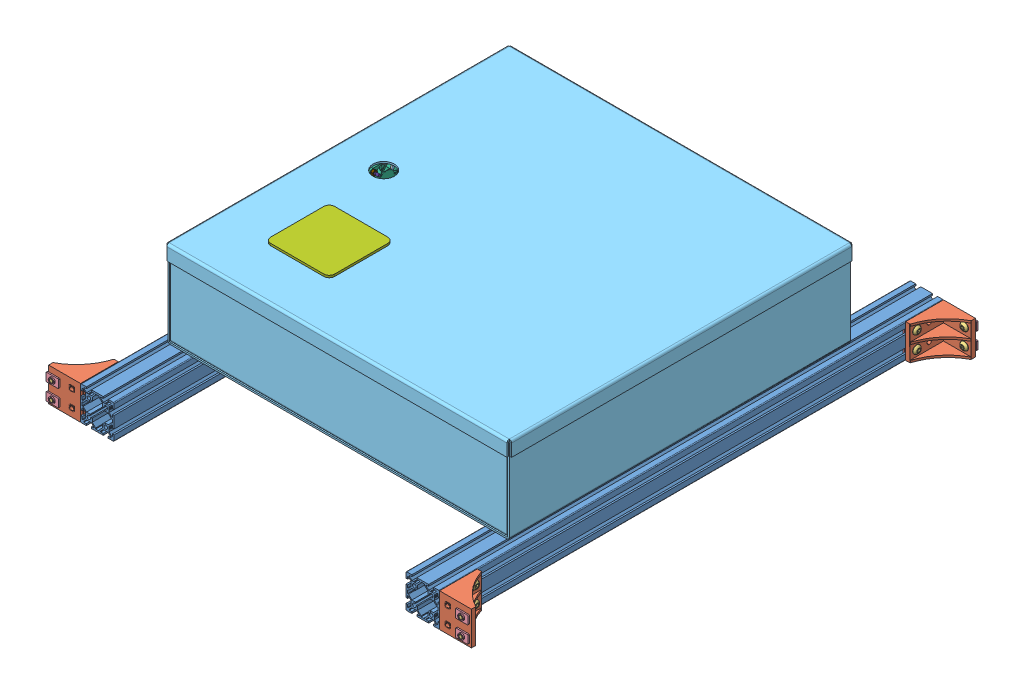
SolidWorks assembly e box uprights, configuration Default. Lengths in mm.
Overall size (503.46 146.17 610.56).
137 component instances, 28 part files, 18 mates.
Components (placement in the parent):
- 4040 600mm-1: 4040 600mm [Default] at (133.4029 328.2364 998.0644) size (40 40 600)
- 4040 600mm-2: 4040 600mm [Default] at (520.8624 328.2364 998.0644) size (40 40 600)
- corner braket assembly-1: corner braket assembly [Default] at (98.8149 314.6768 215.5379) x (0 -1 0) z (-1 0 0) size (40 50.28 43.28)
  - _HBLFSDW5h5_2-1: _HBLFSDW5h5_2 [Default] at (-13.5596 -17.4734 -14.588) size (40 45.8 38.8)
  - 91239A224_CLASS 10.9 STL BUTTON-HEAD SOCKET CAP SCREW-1: 91239A224_CLASS 10.9 STL BUTTON-HEAD SOCKET CAP SCREW [91239A224] at (-23.5596 19.5266 -6.838) size (9.5 9.5 13.21)
  - 91239A224_CLASS 10.9 STL BUTTON-HEAD SOCKET CAP SCREW-3: 91239A224_CLASS 10.9 STL BUTTON-HEAD SOCKET CAP SCREW [91239A224] at (-3.5596 19.5266 -6.838) size (9.5 9.5 13.21)
  - 91239A224_CLASS 10.9 STL BUTTON-HEAD SOCKET CAP SCREW-5: 91239A224_CLASS 10.9 STL BUTTON-HEAD SOCKET CAP SCREW [91239A224] at (-3.5596 -9.7234 15.412) x (1 0 0) z (0 1 0) size (9.5 9.5 13.21)
  - 91239A224_CLASS 10.9 STL BUTTON-HEAD SOCKET CAP SCREW-6: 91239A224_CLASS 10.9 STL BUTTON-HEAD SOCKET CAP SCREW [91239A224] at (-23.5596 -9.7234 15.412) x (1 0 0) z (0 1 0) size (9.5 9.5 13.21)
  - HNKK5-5-2: HNKK5-5 [Default] at (-23.5596 19.5266 -16.588) x (0 0 1) z (0 -1 0) size (3 10 15)
  - HNKK5-5-4: HNKK5-5 [Default] at (-3.5596 19.5266 -16.588) x (0 0 1) z (0 -1 0) size (3 10 15)
  - HNKK5-5-5: HNKK5-5 [Default] at (-23.5596 -19.4734 15.412) x (0 1 0) z (0 0 1) size (3 10 15)
  - HNKK5-5-6: HNKK5-5 [Default] at (-3.5596 -19.4734 15.412) x (0 1 0) z (0 0 1) size (3 10 15)
- corner braket assembly-2: corner braket assembly [Default] at (98.8149 341.796 780.591) x (0 1 0) z (-1 0 0) size (40 50.28 43.28)
  - _HBLFSDW5h5_2-1: _HBLFSDW5h5_2 [Default] at (-13.5596 -17.4734 -14.588) size (40 45.8 38.8)
  - 91239A224_CLASS 10.9 STL BUTTON-HEAD SOCKET CAP SCREW-1: 91239A224_CLASS 10.9 STL BUTTON-HEAD SOCKET CAP SCREW [91239A224] at (-23.5596 19.5266 -6.838) size (9.5 9.5 13.21)
  - 91239A224_CLASS 10.9 STL BUTTON-HEAD SOCKET CAP SCREW-3: 91239A224_CLASS 10.9 STL BUTTON-HEAD SOCKET CAP SCREW [91239A224] at (-3.5596 19.5266 -6.838) size (9.5 9.5 13.21)
  - 91239A224_CLASS 10.9 STL BUTTON-HEAD SOCKET CAP SCREW-5: 91239A224_CLASS 10.9 STL BUTTON-HEAD SOCKET CAP SCREW [91239A224] at (-3.5596 -9.7234 15.412) x (1 0 0) z (0 1 0) size (9.5 9.5 13.21)
  - 91239A224_CLASS 10.9 STL BUTTON-HEAD SOCKET CAP SCREW-6: 91239A224_CLASS 10.9 STL BUTTON-HEAD SOCKET CAP SCREW [91239A224] at (-23.5596 -9.7234 15.412) x (1 0 0) z (0 1 0) size (9.5 9.5 13.21)
  - HNKK5-5-2: HNKK5-5 [Default] at (-23.5596 19.5266 -16.588) x (0 0 1) z (0 -1 0) size (3 10 15)
  - HNKK5-5-4: HNKK5-5 [Default] at (-3.5596 19.5266 -16.588) x (0 0 1) z (0 -1 0) size (3 10 15)
  - HNKK5-5-5: HNKK5-5 [Default] at (-23.5596 -19.4734 15.412) x (0 1 0) z (0 0 1) size (3 10 15)
  - HNKK5-5-6: HNKK5-5 [Default] at (-3.5596 -19.4734 15.412) x (0 1 0) z (0 0 1) size (3 10 15)
- corner braket assembly-3: corner braket assembly [Default] at (555.4504 341.796 215.5379) x (0 1 0) z (1 0 0) size (40 50.28 43.28)
  - _HBLFSDW5h5_2-1: _HBLFSDW5h5_2 [Default] at (-13.5596 -17.4734 -14.588) size (40 45.8 38.8)
  - 91239A224_CLASS 10.9 STL BUTTON-HEAD SOCKET CAP SCREW-1: 91239A224_CLASS 10.9 STL BUTTON-HEAD SOCKET CAP SCREW [91239A224] at (-23.5596 19.5266 -6.838) size (9.5 9.5 13.21)
  - 91239A224_CLASS 10.9 STL BUTTON-HEAD SOCKET CAP SCREW-3: 91239A224_CLASS 10.9 STL BUTTON-HEAD SOCKET CAP SCREW [91239A224] at (-3.5596 19.5266 -6.838) size (9.5 9.5 13.21)
  - 91239A224_CLASS 10.9 STL BUTTON-HEAD SOCKET CAP SCREW-5: 91239A224_CLASS 10.9 STL BUTTON-HEAD SOCKET CAP SCREW [91239A224] at (-3.5596 -9.7234 15.412) x (1 0 0) z (0 1 0) size (9.5 9.5 13.21)
  - 91239A224_CLASS 10.9 STL BUTTON-HEAD SOCKET CAP SCREW-6: 91239A224_CLASS 10.9 STL BUTTON-HEAD SOCKET CAP SCREW [91239A224] at (-23.5596 -9.7234 15.412) x (1 0 0) z (0 1 0) size (9.5 9.5 13.21)
  - HNKK5-5-2: HNKK5-5 [Default] at (-23.5596 19.5266 -16.588) x (0 0 1) z (0 -1 0) size (3 10 15)
  - HNKK5-5-4: HNKK5-5 [Default] at (-3.5596 19.5266 -16.588) x (0 0 1) z (0 -1 0) size (3 10 15)
  - HNKK5-5-5: HNKK5-5 [Default] at (-23.5596 -19.4734 15.412) x (0 1 0) z (0 0 1) size (3 10 15)
  - HNKK5-5-6: HNKK5-5 [Default] at (-3.5596 -19.4734 15.412) x (0 1 0) z (0 0 1) size (3 10 15)
- corner braket assembly-4: corner braket assembly [Default] at (555.4504 314.6768 780.591) x (0 -1 0) z (1 0 0) size (40 50.28 43.28)
  - _HBLFSDW5h5_2-1: _HBLFSDW5h5_2 [Default] at (-13.5596 -17.4734 -14.588) size (40 45.8 38.8)
  - 91239A224_CLASS 10.9 STL BUTTON-HEAD SOCKET CAP SCREW-1: 91239A224_CLASS 10.9 STL BUTTON-HEAD SOCKET CAP SCREW [91239A224] at (-23.5596 19.5266 -6.838) size (9.5 9.5 13.21)
  - 91239A224_CLASS 10.9 STL BUTTON-HEAD SOCKET CAP SCREW-3: 91239A224_CLASS 10.9 STL BUTTON-HEAD SOCKET CAP SCREW [91239A224] at (-3.5596 19.5266 -6.838) size (9.5 9.5 13.21)
  - 91239A224_CLASS 10.9 STL BUTTON-HEAD SOCKET CAP SCREW-5: 91239A224_CLASS 10.9 STL BUTTON-HEAD SOCKET CAP SCREW [91239A224] at (-3.5596 -9.7234 15.412) x (1 0 0) z (0 1 0) size (9.5 9.5 13.21)
  - 91239A224_CLASS 10.9 STL BUTTON-HEAD SOCKET CAP SCREW-6: 91239A224_CLASS 10.9 STL BUTTON-HEAD SOCKET CAP SCREW [91239A224] at (-23.5596 -9.7234 15.412) x (1 0 0) z (0 1 0) size (9.5 9.5 13.21)
  - HNKK5-5-2: HNKK5-5 [Default] at (-23.5596 19.5266 -16.588) x (0 0 1) z (0 -1 0) size (3 10 15)
  - HNKK5-5-4: HNKK5-5 [Default] at (-3.5596 19.5266 -16.588) x (0 0 1) z (0 -1 0) size (3 10 15)
  - HNKK5-5-5: HNKK5-5 [Default] at (-23.5596 -19.4734 15.412) x (0 1 0) z (0 0 1) size (3 10 15)
  - HNKK5-5-6: HNKK5-5 [Default] at (-3.5596 -19.4734 15.412) x (0 1 0) z (0 0 1) size (3 10 15)
- elc box assebly-1: elc box assebly [Default] at (129.7196 154.3271 230.9368) size (410.46 106.17 430.94)
  - Electrical Enclosure 16 in-1: Electrical Enclosure 16 in [Default] at (-5.7869 193.9093 67.1276) size (410.46 103.63 410.46)
  - elc component panel-1: elc component panel [Default] at (423.6423 -1.464 537.2069) x (-1 0 0) z (0 0 -1) size (369.37 85.56 330.2)
    - elc plate-1: elc plate [Default] at (226.2293 207.4053 266.8793) size (368.3 1.59 330.2)
    - power supply with standoffs-1: power supply with standoffs [Default] at (35.6304 133.9192 294.786) x (0 0 -1) z (1 0 0) size (115.2 58.27 215)
      - __-1: __ [По умолчанию] at (110.1067 83.0736 152.0488) size (115.2 50.11 215)
      - 95783A055_NYLON 6 6 MALE-FEMALE THREADED HEX STANDOFF-1: 95783A055_NYLON 6 6 MALE-FEMALE THREADED HEX STANDOFF [95783A055] at (85.1067 81.4236 77.0488) x (0 1 0) z (0 0 1) size (13.03 5.2 4.5)
      - 95783A055_NYLON 6 6 MALE-FEMALE THREADED HEX STANDOFF-2: 95783A055_NYLON 6 6 MALE-FEMALE THREADED HEX STANDOFF [95783A055] at (135.1067 81.4236 77.0488) x (0 1 0) z (-0.939028 0 -0.343839) size (13.03 5.2 4.5)
      - 95783A055_NYLON 6 6 MALE-FEMALE THREADED HEX STANDOFF-3: 95783A055_NYLON 6 6 MALE-FEMALE THREADED HEX STANDOFF [95783A055] at (135.1067 81.4236 227.0488) x (0 1 0) z (-0.996262 0 -0.086381) size (13.03 5.2 4.5)
      - 95783A055_NYLON 6 6 MALE-FEMALE THREADED HEX STANDOFF-4: 95783A055_NYLON 6 6 MALE-FEMALE THREADED HEX STANDOFF [95783A055] at (85.1067 81.4236 227.0488) x (0 1 0) z (-0.990494 0 -0.137554) size (13.03 5.2 4.5)
    - arduino board assembly-1: arduino board assembly [Default] at (260.6228 173.6976 405.5467) x (0 0 -1) z (1 0 0) size (100 30.86 52.88)
      - ArduinoMega2560 CORRECTED-1: ArduinoMega2560 CORRECTED [Default] at (48.9673 43.2952 72.715) size (100 11.65 51.63)
      - breakout board-1: breakout board [Default] at (48.9673 54.2952 72.715) size (100 7 51.63)
      - 95783A055_NYLON 6 6 MALE-FEMALE THREADED HEX STANDOFF-1: 95783A055_NYLON 6 6 MALE-FEMALE THREADED HEX STANDOFF [95783A055] at (84.2031 36.9452 49.5995) x (0 -1 0) z (0 0 1) size (13.03 5.2 4.5)
      - 95783A055_NYLON 6 6 MALE-FEMALE THREADED HEX STANDOFF-2: 95783A055_NYLON 6 6 MALE-FEMALE THREADED HEX STANDOFF [95783A055] at (3.483 36.9452 49.7272) x (0 -1 0) z (0 0 1) size (13.03 5.2 4.5)
      - 95783A055_NYLON 6 6 MALE-FEMALE THREADED HEX STANDOFF-3: 95783A055_NYLON 6 6 MALE-FEMALE THREADED HEX STANDOFF [95783A055] at (9.6911 36.9452 96.9805) x (0 -1 0) z (0 0 1) size (13.03 5.2 4.5)
      - 91290A110_BLACK-OXIDE CLASS 12.9 SOCKET HEAD CAP SCREW-1: 91290A110_BLACK-OXIDE CLASS 12.9 SOCKET HEAD CAP SCREW [91290A110] at (9.6911 39.2952 96.9805) x (1 0 0) z (0 -1 0) size (5.5 5.5 8.18)
      - 91290A110_BLACK-OXIDE CLASS 12.9 SOCKET HEAD CAP SCREW-2: 91290A110_BLACK-OXIDE CLASS 12.9 SOCKET HEAD CAP SCREW [91290A110] at (84.2031 39.2952 49.5995) x (1 0 0) z (0 -1 0) size (5.5 5.5 8.18)
      - 91290A110_BLACK-OXIDE CLASS 12.9 SOCKET HEAD CAP SCREW-3: 91290A110_BLACK-OXIDE CLASS 12.9 SOCKET HEAD CAP SCREW [91290A110] at (3.483 39.2952 49.7272) x (1 0 0) z (0 -1 0) size (5.5 5.5 8.18)
    - din rail assmbly-1: din rail assmbly [Default] at (226.6874 101.8607 473.572) x (-1 0 0) z (0 0 -1) size (90.31 80.69 125)
      - DIN 59_0-1: DIN 59_0 [00] at (103.6081 107.1321 54.2926) size (35 7.5 125)
      - SEIMENS 8WA1 808 DIN RAIL END RETAINER-1: SEIMENS 8WA1 808 DIN RAIL END RETAINER [Default] at (102.6081 107.6321 71.2884) size (45 44.95 10)
      - SEIMENS 8WA1 808 DIN RAIL END RETAINER-3: SEIMENS 8WA1 808 DIN RAIL END RETAINER [Default] at (102.6081 107.6321 162.4924) size (45 44.95 10)
      - 3812830-8: 3812830 [Default] at (102.7638 140.3713 56.6988) x (0 0 -1) z (1 0 0) size (6.2 76.69 90.31)
        - 3812830A-1: 3812830A [Default] at (-75.9936 -29.2392 18.3443) size (6.2 76.69 90.31)
        - 3812830B-1: 3812830B [Default] at (-75.3936 25.9608 19.6) size (5 19.3 28)
      - 3812830-9: 3812830 [Default] at (102.7638 140.3713 62.8988) x (0 0 -1) z (1 0 0) size (6.2 76.69 90.31)
        - 3812830A-1: 3812830A [Default] at (-75.9936 -29.2392 18.3443) size (6.2 76.69 90.31)
        - 3812830B-1: 3812830B [Default] at (-75.3936 25.9608 19.6) size (5 19.3 28)
      - 3812830-10: 3812830 [Default] at (102.7638 140.3713 69.0988) x (0 0 -1) z (1 0 0) size (6.2 76.69 90.31)
        - 3812830A-1: 3812830A [Default] at (-75.9936 -29.2392 18.3443) size (6.2 76.69 90.31)
        - 3812830B-1: 3812830B [Default] at (-75.3936 25.9608 19.6) size (5 19.3 28)
      - 3812830-11: 3812830 [Default] at (102.7638 140.3713 75.2988) x (0 0 -1) z (1 0 0) size (6.2 76.69 90.31)
        - 3812830A-1: 3812830A [Default] at (-75.9936 -29.2392 18.3443) size (6.2 76.69 90.31)
        - 3812830B-1: 3812830B [Default] at (-75.3936 25.9608 19.6) size (5 19.3 28)
      - 3812830-12: 3812830 [Default] at (102.7638 140.3713 81.4988) x (0 0 -1) z (1 0 0) size (6.2 76.69 90.31)
        - 3812830A-1: 3812830A [Default] at (-75.9936 -29.2392 18.3443) size (6.2 76.69 90.31)
        - 3812830B-1: 3812830B [Default] at (-75.3936 25.9608 19.6) size (5 19.3 28)
      - Din fuse-1: Din fuse [Default] at (59.9389 109.5521 90.7664) size (82.55 57.15 9.65)
      - Din fuse-2: Din fuse [Default] at (59.9389 109.5521 81.1144) size (82.55 57.15 9.65)
      - dinrail_Terminal-11: dinrail_Terminal [Default] at (121.1081 114.6321 95.5924) size (48 46.85 5.15)
      - dinrail_Terminal-12: dinrail_Terminal [Default] at (121.1081 114.6321 100.7424) size (48 46.85 5.15)
      - dinrail_Terminal-13: dinrail_Terminal [Default] at (121.1081 114.6321 111.0424) size (48 46.85 5.15)
      - dinrail_Terminal-16: dinrail_Terminal [Default] at (121.1081 114.6321 105.8924) size (48 46.85 5.15)
      - dinrail_Terminal-17: dinrail_Terminal [Default] at (121.1081 114.6321 116.1924) size (48 46.85 5.15)
      - dinrail_Terminal-18: dinrail_Terminal [Default] at (121.1081 114.6321 121.3424) size (48 46.85 5.15)
    - arduino board assembly-2: arduino board assembly [Default] at (164.5922 173.6976 405.5467) x (0 0 -1) z (1 0 0) size (100 30.86 52.88)
      - ArduinoMega2560 CORRECTED-1: ArduinoMega2560 CORRECTED [Default] at (48.9673 43.2952 72.715) size (100 11.65 51.63)
      - breakout board-1: breakout board [Default] at (48.9673 54.2952 72.715) size (100 7 51.63)
      - 95783A055_NYLON 6 6 MALE-FEMALE THREADED HEX STANDOFF-1: 95783A055_NYLON 6 6 MALE-FEMALE THREADED HEX STANDOFF [95783A055] at (84.2031 36.9452 49.5995) x (0 -1 0) z (0 0 1) size (13.03 5.2 4.5)
      - 95783A055_NYLON 6 6 MALE-FEMALE THREADED HEX STANDOFF-2: 95783A055_NYLON 6 6 MALE-FEMALE THREADED HEX STANDOFF [95783A055] at (3.483 36.9452 49.7272) x (0 -1 0) z (0 0 1) size (13.03 5.2 4.5)
      - 95783A055_NYLON 6 6 MALE-FEMALE THREADED HEX STANDOFF-3: 95783A055_NYLON 6 6 MALE-FEMALE THREADED HEX STANDOFF [95783A055] at (9.6911 36.9452 96.9805) x (0 -1 0) z (0 0 1) size (13.03 5.2 4.5)
      - 91290A110_BLACK-OXIDE CLASS 12.9 SOCKET HEAD CAP SCREW-1: 91290A110_BLACK-OXIDE CLASS 12.9 SOCKET HEAD CAP SCREW [91290A110] at (9.6911 39.2952 96.9805) x (1 0 0) z (0 -1 0) size (5.5 5.5 8.18)
      - 91290A110_BLACK-OXIDE CLASS 12.9 SOCKET HEAD CAP SCREW-2: 91290A110_BLACK-OXIDE CLASS 12.9 SOCKET HEAD CAP SCREW [91290A110] at (84.2031 39.2952 49.5995) x (1 0 0) z (0 -1 0) size (5.5 5.5 8.18)
      - 91290A110_BLACK-OXIDE CLASS 12.9 SOCKET HEAD CAP SCREW-3: 91290A110_BLACK-OXIDE CLASS 12.9 SOCKET HEAD CAP SCREW [91290A110] at (3.483 39.2952 49.7272) x (1 0 0) z (0 -1 0) size (5.5 5.5 8.18)
    - 92497A200_ZINC YELLOW-CHROMATE PLATED STEEL HEX NUT-1: 92497A200_ZINC YELLOW-CHROMATE PLATED STEEL HEX NUT [92497A200] at (214.3194 206.2053 402.0637) x (1 0 0) z (0 1 0) size (5.5 6.35 2.78)
    - 92497A200_ZINC YELLOW-CHROMATE PLATED STEEL HEX NUT-2: 92497A200_ZINC YELLOW-CHROMATE PLATED STEEL HEX NUT [92497A200] at (214.1917 206.2053 321.3436) x (1 0 0) z (0 1 0) size (5.5 6.35 2.78)
    - 92497A200_ZINC YELLOW-CHROMATE PLATED STEEL HEX NUT-3: 92497A200_ZINC YELLOW-CHROMATE PLATED STEEL HEX NUT [92497A200] at (261.5727 206.2053 395.8556) x (1 0 0) z (0 1 0) size (5.5 6.35 2.78)
    - 92497A200_ZINC YELLOW-CHROMATE PLATED STEEL HEX NUT-4: 92497A200_ZINC YELLOW-CHROMATE PLATED STEEL HEX NUT [92497A200] at (310.3501 206.2053 402.0637) x (1 0 0) z (0 1 0) size (5.5 6.35 2.78)
    - 92497A200_ZINC YELLOW-CHROMATE PLATED STEEL HEX NUT-5: 92497A200_ZINC YELLOW-CHROMATE PLATED STEEL HEX NUT [92497A200] at (310.2224 206.2053 321.3436) x (1 0 0) z (0 1 0) size (5.5 6.35 2.78)
    - 92497A200_ZINC YELLOW-CHROMATE PLATED STEEL HEX NUT-6: 92497A200_ZINC YELLOW-CHROMATE PLATED STEEL HEX NUT [92497A200] at (357.6034 206.2053 395.8556) x (1 0 0) z (0 1 0) size (5.5 6.35 2.78)
    - 92095A177_18-8 SS BUTTON-HEAD SOCKET CAP SCREW-1: 92095A177_18-8 SS BUTTON-HEAD SOCKET CAP SCREW [92095A177] at (262.6793 205.7553 159.6793) x (1 0 0) z (0 -1 0) size (5.7 5.7 6.94)
    - 92095A177_18-8 SS BUTTON-HEAD SOCKET CAP SCREW-3: 92095A177_18-8 SS BUTTON-HEAD SOCKET CAP SCREW [92095A177] at (112.6793 205.7553 159.6793) x (1 0 0) z (0 -1 0) size (5.7 5.7 6.94)
    - 92095A177_18-8 SS BUTTON-HEAD SOCKET CAP SCREW-4: 92095A177_18-8 SS BUTTON-HEAD SOCKET CAP SCREW [92095A177] at (112.6793 205.7553 209.6793) x (1 0 0) z (0 -1 0) size (5.7 5.7 6.94)
    - small panduit 1-2: small panduit 1 [Default] at (435.7793 210.2628 274.3593) size (368.3 30.38 16.31)
    - small panduit 4-6: small panduit 4 [Default] at (286.3538 210.2628 21.6293) x (0 0 -1) z (1 0 0) size (133.35 30.38 16.31)
    - small panduit 4-7: small panduit 4 [Default] at (188.9955 210.2628 21.6293) x (0 0 -1) z (1 0 0) size (133.35 30.38 16.31)
    - small panduit 4-8: small panduit 4 [Default] at (325.6017 210.2628 527.0893) x (0 0 1) z (-1 0 0) size (133.35 30.38 16.31)
    - small panduit 3-2: small panduit 3 [Default] at (541.8293 210.2628 422.9493) size (222.25 30.38 16.31)
    - small panduit 2-10: small panduit 2 [Default] at (49.6993 210.2628 -3.7707) x (0 0 -1) z (1 0 0) size (107.95 30.38 16.31)
    - small panduit 2-11: small panduit 2 [Default] at (402.7593 210.2628 -3.7707) x (0 0 -1) z (1 0 0) size (107.95 30.38 16.31)
  - 40x40x10 DC Fan-1: 40x40x10 DC Fan [Default] at (249.8006 244.7093 74.4096) size (49.86 40.69 10.5)
  - 40x40x10 DC Fan-2: 40x40x10 DC Fan [Default] at (1.4951 244.7093 225.8776) x (0 0 -1) z (1 0 0) size (49.86 40.69 10.5)
  - fan hole cover-1: fan hole cover [Default] at (90.1997 300.0813 377.5156) x (-1 0 0) z (0 0 1) size (76.2 12.7 76.2)
  - 92095A185_18-8 SS BUTTON-HEAD SOCKET CAP SCREW-1: 92095A185_18-8 SS BUTTON-HEAD SOCKET CAP SCREW [92095A185] at (265.8026 260.7113 65.4776) x (-0.923728 -0.383049 0) z (0 0 -1) size (5.7 5.7 22.02)
  - 92095A185_18-8 SS BUTTON-HEAD SOCKET CAP SCREW-2: 92095A185_18-8 SS BUTTON-HEAD SOCKET CAP SCREW [92095A185] at (233.7986 228.7073 65.4776) x (-0.923728 -0.383049 0) z (0 0 -1) size (5.7 5.7 22.02)
  - 92095A185_18-8 SS BUTTON-HEAD SOCKET CAP SCREW-3: 92095A185_18-8 SS BUTTON-HEAD SOCKET CAP SCREW [92095A185] at (-7.4369 260.7113 241.8796) x (0 0 1) z (-1 0 0) size (5.7 5.7 22.02)
  - 92095A185_18-8 SS BUTTON-HEAD SOCKET CAP SCREW-4: 92095A185_18-8 SS BUTTON-HEAD SOCKET CAP SCREW [92095A185] at (-7.4369 228.7073 209.8756) x (0 0 1) z (-1 0 0) size (5.7 5.7 22.02)
  - 92497A200_ZINC YELLOW-CHROMATE PLATED STEEL HEX NUT-1: 92497A200_ZINC YELLOW-CHROMATE PLATED STEEL HEX NUT [92497A200] at (265.8006 260.7093 80.8596) size (5.5 6.35 2.78)
  - 92497A200_ZINC YELLOW-CHROMATE PLATED STEEL HEX NUT-2: 92497A200_ZINC YELLOW-CHROMATE PLATED STEEL HEX NUT [92497A200] at (233.8006 228.7093 80.8596) size (5.5 6.35 2.78)
  - 92497A200_ZINC YELLOW-CHROMATE PLATED STEEL HEX NUT-3: 92497A200_ZINC YELLOW-CHROMATE PLATED STEEL HEX NUT [92497A200] at (7.9451 228.7093 209.8776) x (0 0 -1) z (1 0 0) size (5.5 6.35 2.78)
  - 92497A200_ZINC YELLOW-CHROMATE PLATED STEEL HEX NUT-4: 92497A200_ZINC YELLOW-CHROMATE PLATED STEEL HEX NUT [92497A200] at (7.9451 260.7093 241.8776) x (0 0 -1) z (1 0 0) size (5.5 6.35 2.78)
  - IEC320-C20-1: IEC320-C20 [Default] at (337.2782 245.1157 67.3026) size (31 24 28.57)
  - gland_m12-1: gland_m12 [Default] at (95.8131 219.3093 75.1276) x (1 0 0) z (0 1 0) size (16.94 30.51 16.89)
  - gland_m12-2: gland_m12 [Default] at (45.0131 219.3093 75.1276) x (1 0 0) z (0 1 0) size (16.94 30.51 16.89)
  - gland_m12-3: gland_m12 [Default] at (70.4131 244.7093 75.1276) x (1 0 0) z (0 1 0) size (16.94 30.51 16.89)
  - gland_m12-4: gland_m12 [Default] at (45.0131 244.7093 75.1276) x (1 0 0) z (0 1 0) size (16.94 30.51 16.89)
  - gland_m12-5: gland_m12 [Default] at (19.6131 244.7093 75.1276) x (1 0 0) z (0 1 0) size (16.94 30.51 16.89)
  - gland_m12-6: gland_m12 [Default] at (45.0131 270.1093 75.1276) x (-0.923728 -0.383049 0) z (0.383049 -0.923728 0) size (16.94 30.51 16.89)
  - gland_m12-7: gland_m12 [Default] at (19.6131 270.1093 75.1276) x (-0.923728 -0.383049 0) z (0.383049 -0.923728 0) size (16.94 30.51 16.89)
  - gland_m12-9: gland_m12 [Default] at (70.4131 219.3093 75.1276) x (1 0 0) z (0 1 0) size (16.94 30.51 16.89)
  - gland_m12-10: gland_m12 [Default] at (19.6131 219.3093 75.1276) x (1 0 0) z (0 1 0) size (16.94 30.51 16.89)
  - gland_m12-11: gland_m12 [Default] at (95.8131 244.7093 75.1276) x (1 0 0) z (0 1 0) size (16.94 30.51 16.89)
  - gland_m12-12: gland_m12 [Default] at (70.4131 270.1093 75.1276) x (1 0 0) z (0 1 0) size (16.94 30.51 16.89)
  - gland_m12-13: gland_m12 [Default] at (95.8131 270.1093 75.1276) x (1 0 0) z (0 1 0) size (16.94 30.51 16.89)
Mates (geometry in assembly coordinates):
- Coincident1: coincident: plane of 4040 600mm-1 through (113.4029 335.2364 198.0644) normal (-1 0 0); plane of corner braket assembly-2/_HBLFSDW5h5_2-1 through (113.4029 328.2364 798.0644) normal (1 0 0)
- Coincident2: coincident: plane of 4040 600mm-1 through (140.4029 348.2364 198.0644) normal (0 1 0); plane of corner braket assembly-2/_HBLFSDW5h5_2-1 through (76.4029 348.2364 793.4237) normal (0 1 0)
- Coincident3: coincident: plane of 4040 600mm-1 through (119.9029 318.89 798.0644) normal (0 0 1); plane of corner braket assembly-2/_HBLFSDW5h5_2-1 through (114.2029 308.2364 798.0644) normal (0 0 1)
- Coincident4: coincident: plane of 4040 600mm-1 through (140.4029 348.2364 198.0644) normal (0 1 0); plane of 4040 600mm-2 through (527.8624 348.2364 198.0644) normal (0 1 0)
- Coincident5: coincident: plane of 4040 600mm-1 through (119.9029 318.89 798.0644) normal (0 0 1); plane of 4040 600mm-2 through (507.3624 318.89 798.0644) normal (0 0 1)
- Coincident6: coincident: plane of 4040 600mm-2 through (540.8624 321.2364 198.0644) normal (1 0 0); plane of corner braket assembly-4/_HBLFSDW5h5_2-1 through (540.8624 328.2364 798.0644) normal (-1 0 0)
- Coincident7: coincident: plane of 4040 600mm-2 through (527.8624 348.2364 198.0644) normal (0 1 0); plane of corner braket assembly-4/_HBLFSDW5h5_2-1 through (577.8624 348.2364 793.4237) normal (0 1 0)
- Coincident8: coincident: plane of 4040 600mm-2 through (507.3624 318.89 798.0644) normal (0 0 1); plane of corner braket assembly-4/_HBLFSDW5h5_2-1 through (540.0624 348.2364 798.0644) normal (0 0 1)
- Coincident9: coincident: plane of 4040 600mm-1 through (113.4029 335.2364 198.0644) normal (-1 0 0); plane of corner braket assembly-1/_HBLFSDW5h5_2-1 through (113.4029 328.2364 198.0644) normal (1 0 0)
- Coincident10: coincident: plane of 4040 600mm-1 through (140.4029 348.2364 198.0644) normal (0 1 0); plane of corner braket assembly-1/_HBLFSDW5h5_2-1 through (76.4029 348.2364 202.7052) normal (0 1 0)
- Coincident11: coincident: plane of 4040 600mm-1 through (119.9029 318.89 198.0644) normal (0 0 -1); plane of corner braket assembly-1/_HBLFSDW5h5_2-1 through (114.2029 348.2364 198.0644) normal (0 0 -1)
- Coincident12: coincident: plane of 4040 600mm-2 through (540.8624 321.2364 198.0644) normal (1 0 0); plane of corner braket assembly-3/_HBLFSDW5h5_2-1 through (540.8624 328.2364 198.0644) normal (-1 0 0)
- Coincident13: coincident: plane of 4040 600mm-2 through (527.8624 348.2364 198.0644) normal (0 1 0); plane of corner braket assembly-3/_HBLFSDW5h5_2-1 through (577.8624 348.2364 202.7052) normal (0 1 0)
- Coincident14: coincident: plane of 4040 600mm-2 through (507.3624 318.89 198.0644) normal (0 0 -1); plane of corner braket assembly-3/_HBLFSDW5h5_2-1 through (540.0624 308.2364 198.0644) normal (0 0 -1)
- Coincident15: coincident: plane of 4040 600mm-1 through (140.4029 348.2364 198.0644) normal (0 1 0); plane of elc box assebly-1/Electrical Enclosure 16 in-1 through (123.9326 348.2364 704.4644) normal (0 -1 0)
- Tangent1: tangent: plane of 4040 600mm-1 through (140.4029 346.2364 198.0644) normal (1 0 0); cylinder of elc box assebly-1/Electrical Enclosure 16 in-1 through (142.9826 348.2364 666.3644) axis (0 -1 0) radius 2.5798
- Tangent2: tangent: plane of 4040 600mm-2 through (513.8624 348.2364 198.0644) normal (-1 0 0); cylinder of elc box assebly-1/Electrical Enclosure 16 in-1 through (511.2826 348.2364 666.3644) axis (0 -1 0) radius 2.5798
- Distance1: distance = 100 mm: plane of elc box assebly-1/Electrical Enclosure 16 in-1 through (123.9326 348.2364 298.0644) normal (0 0 -1); plane of 4040 600mm-1 through (119.9029 318.89 198.0644) normal (0 0 -1)
